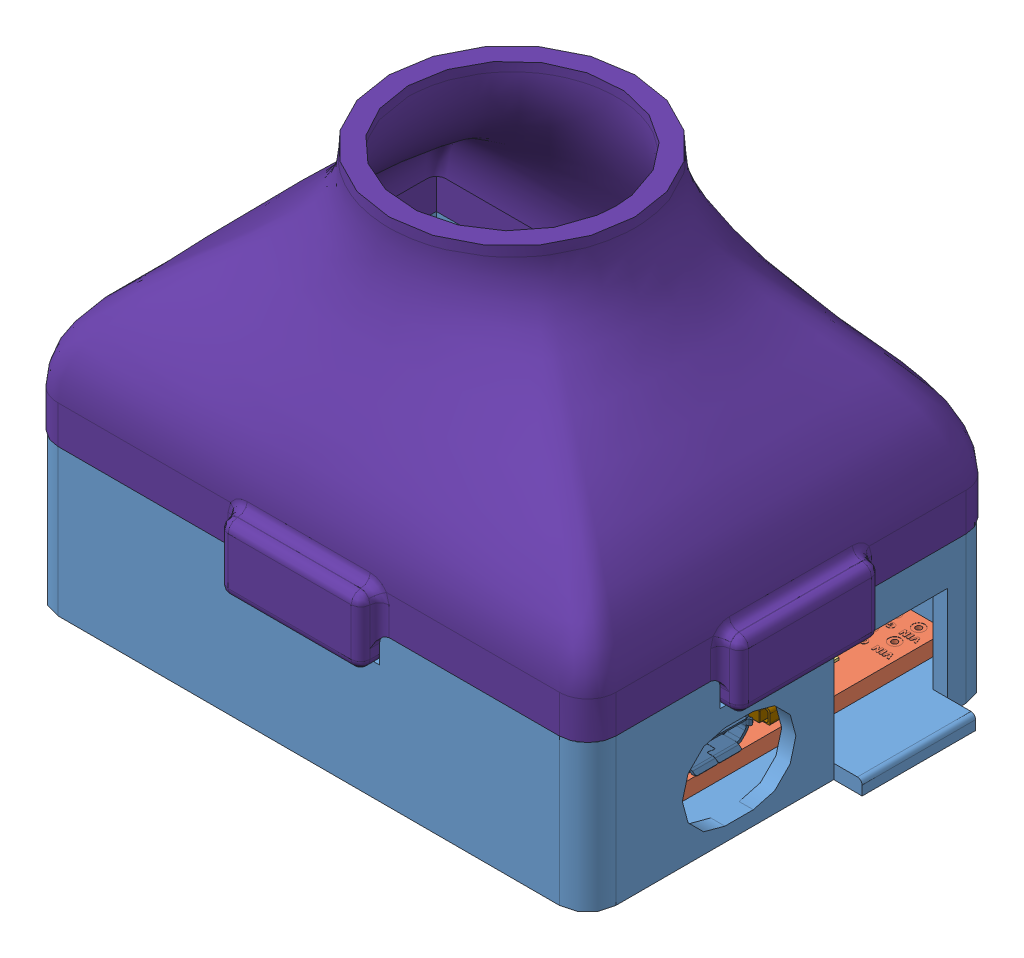
SolidWorks assembly Arduino Case Assembly, configuration Default. Lengths in mm.
Overall size (73 45.5 47).
47 component instances, 17 part files, 8 mates.
Components (placement in the parent):
- Mega 2560 Pro embed Case-1: Mega 2560 Pro embed Case [Default] at origin size (73 15.5 43)
- MEGA 2560 PRO (EMBED)-1: MEGA 2560 PRO (EMBED) [Default] at (0 3.5 0) x (0 0 1) z (0 1 0) size (38 54.09 6.02)
  - MEGA 2560 PRO (EMBED).stp-1: MEGA 2560 PRO (EMBED).stp [Default] at origin size (38 54.09 6.02)
    - Mega 2560 Pro - Board.stp-1: Mega 2560 Pro - Board.stp [Default] at origin size (38 54 1.78)
    - SOT223-3.stp-1: SOT223-3.stp [Default] at (-7.7036 13.3224 1.6256) x (-1 0 0) z (0 0 1) size (6.5 7.07 1.6)
    - SOT223-3.stp-2: SOT223-3.stp [Default] at (-7.5781 23.9617 1.6256) x (-1 0 0) z (0 0 1) size (6.5 7.07 1.6)
    - ATmega2560-16AU.stp-1: ATmega2560-16AU.stp [Default] at (0.2253 -9.3836 1.5256) x (0.707107 -0.707107 0) z (0 0 1) size (16 16 1.21)
    - SOIC -16.stp-1: SOIC -16.stp [Default] at (0.546 8.9647 1.4756) x (0 1 0) z (1 0 0) size (6 1.4 9.9)
    - Crystal Oscillator (SMD).stp-1: Crystal Oscillator (SMD).stp [Default] at (-10.7852 -19.6364 2.54) x (0 -1 0) z (0 0 1) size (13.06 4.55 4.32)
    - Crystal Oscillator (SMD).stp-2: Crystal Oscillator (SMD).stp [Default] at (10.6809 3.6875 2.54) x (0 -1 0) z (0 0 1) size (13.06 4.55 4.32)
    - 1206 Capacitor.stp-1: 1206 Capacitor.stp [Default] at (-3.8106 17.9279 1.6231) x (0 -1 0) z (0 0 1) size (3.2 1.6 1.6)
    - Fuse (1206) - Green.stp-1: Fuse (1206) - Green.stp [Default] at (-0.2207 16.3875 1.6281) x (0 -1 0) z (0 0 1) size (3.28 1.75 0.87)
    - Diode - SMD - DO-214AC.stp-1: Diode - SMD - DO-214AC.stp [Default] at (-1.7706 25.543 1.4756) x (0 -1 0) z (0 0 1) size (5.6 2.95 2.91)
    - USB - Micro.stp-1: USB - Micro.stp [Default] at (2.2104 21.1734 1.3475) x (-1 0 0) z (0 1 0) size (7.92 3.01 5.67)
    - 0603 Capacitor.stp-1: 0603 Capacitor.stp [Default] at (10.7145 18.9901 1.6231) x (0 -1 0) z (0 0 1) size (1.6 0.84 0.84)
    - 0603 Capacitor.stp-2: 0603 Capacitor.stp [Default] at (4.611 3.4374 1.6231) x (0 -1 0) z (0 0 1) size (1.6 0.84 0.84)
    - 0603 Capacitor.stp-3: 0603 Capacitor.stp [Default] at (7.1573 7.8647 1.6231) x (0 1 0) z (0 0 1) size (1.6 0.84 0.84)
    - 0603 Capacitor.stp-4: 0603 Capacitor.stp [Default] at (7.0977 13.4599 1.6231) x (0 1 0) z (0 0 1) size (1.6 0.84 0.84)
    - 0603 Capacitor.stp-5: 0603 Capacitor.stp [Default] at (5.1576 -19.4722 1.6231) x (0 1 0) z (1 0 0) size (1.6 0.84 0.84)
    - 0603 Capacitor.stp-6: 0603 Capacitor.stp [Default] at (-10.8858 1.8771 1.6231) x (0 1 0) z (1 0 0) size (1.6 0.84 0.84)
    - 0603 Capacitor.stp-7: 0603 Capacitor.stp [Default] at (2.9599 3.4697 1.6231) x (0 -1 0) z (0 0 1) size (1.6 0.84 0.84)
    - 0603 Capacitor.stp-8: 0603 Capacitor.stp [Default] at (2.0157 3.7447 1.6231) x (-1 0 0) z (0 0 1) size (1.6 0.84 0.84)
    - 0603 Capacitor.stp-9: 0603 Capacitor.stp [Default] at (-8.0885 -1.9063 1.6231) x (0 1 0) z (1 0 0) size (1.6 0.84 0.84)
    - 0603 Capacitor.stp-10: 0603 Capacitor.stp [Default] at (-3.7884 20.5934 1.6231) x (0 1 0) z (0 0 1) size (1.6 0.84 0.84)
    - 0603 Capacitor.stp-11: 0603 Capacitor.stp [Default] at (-8.8216 3.4762 1.6231) x (0 -1 0) z (0 0 1) size (1.6 0.84 0.84)
    - 0603 Capacitor.stp-12: 0603 Capacitor.stp [Default] at (6.3032 3.4697 2.4613) x (0 -1 0) z (1 0 0) size (1.6 0.84 0.84)
    - 0603 Capacitor.stp-13: 0603 Capacitor.stp [Default] at (-6.2819 -20.9115 1.6231) x (-1 0 0) z (0 1 0) size (1.6 0.84 0.84)
    - 0603 Capacitor.stp-14: 0603 Capacitor.stp [Default] at (-7.8888 -17.889 1.6231) size (1.6 0.84 0.84)
    - 0603 Resistor.stp-1: 0603 Resistor.stp [Default] at (-6.1185 1.9325 1.6231) x (0 1 0) z (0 0 1) size (1.6 0.85 0.56)
    - 0603 Resistor.stp-2: 0603 Resistor.stp [Default] at (-8.697 -1.8307 1.6231) x (0 1 0) z (0 0 1) size (1.6 0.85 0.56)
    - 0603 Resistor.stp-3: 0603 Resistor.stp [Default] at (-10.3133 -1.7908 1.6231) x (0 1 0) z (0 0 1) size (1.6 0.85 0.56)
    - 0603 Resistor.stp-4: 0603 Resistor.stp [Default] at (6.8981 17.2332 1.6231) x (0 1 0) z (0 0 1) size (1.6 0.85 0.56)
    - 0603 Resistor.stp-5: 0603 Resistor.stp [Default] at (-4.1536 1.9449 1.6231) x (0 1 0) z (0 0 1) size (1.6 0.85 0.56)
    - 0603 Resistor.stp-6: 0603 Resistor.stp [Default] at (7.1292 10.6782 1.6231) x (0 1 0) z (0 0 1) size (1.6 0.85 0.56)
    - 0603 Resistor.stp-7: 0603 Resistor.stp [Default] at (5.2754 17.2903 1.6231) x (0 1 0) z (0 0 1) size (1.6 0.85 0.56)
    - 0603 Resistor.stp-8: 0603 Resistor.stp [Default] at (9.8818 17.3443 1.6231) x (0 1 0) z (0 0 1) size (1.6 0.85 0.56)
    - 0603 Resistor.stp-9: 0603 Resistor.stp [Default] at (-11.9263 1.9088 1.6231) x (0 1 0) z (0 0 1) size (1.6 0.85 0.56)
    - 0603 Resistor.stp-10: 0603 Resistor.stp [Default] at (7.18 4.9009 1.6231) x (0 1 0) z (0 0 1) size (1.6 0.85 0.56)
    - 0603 Resistor.stp-11: 0603 Resistor.stp [Default] at (-11.9146 -1.6797 1.6231) x (0 1 0) z (0 0 1) size (1.6 0.85 0.56)
    - 0603 Resistor.stp-12: 0603 Resistor.stp [Default] at (-6.3495 -18.5603 1.6231) x (-1 0 0) z (0 0 1) size (1.6 0.85 0.56)
    - LED - 0603 - Blue.stp-1: LED - 0603 - Blue.stp [Default] at (7.1908 -19.2239 1.6256) x (0 1 0) z (0 0 1) size (1.63 0.73 0.83)
    - LED_-_Vishay_-_6063_-_Green.stp-1: LED_-_Vishay_-_6063_-_Green.stp [Default] at (10.6783 -18.0475 1.5956) x (0 -1 0) z (0 0 1) size (1.63 0.73 0.83)
    - LED - 0603 - Blue.stp-2: LED - 0603 - Blue.stp [Default] at (9.0246 -17.9783 1.6256) x (0 -1 0) z (0 0 1) size (1.63 0.73 0.83)
    - 1206 Fuse.stp-1: 1206 Fuse.stp [Default] at (1.6964 17.9461 1.6231) x (0 -1 0) z (0 0 1) size (3.2 1.6 0.53)
    - SWT-32.stp-1: SWT-32.stp [Default] at (15.7781 21.6695 1.6256) x (0 1 0) z (0 0 1) size (8 6.4 2.9)
    - LED - 0603 - Blue.stp-3: LED - 0603 - Blue.stp [Default] at (12.5463 -18.1103 1.6256) x (0 -1 0) z (0 0 1) size (1.63 0.73 0.83)
- Arduino cables-1: Arduino cables [Default] at (0 15.5 0) x (1 0 0) z (0 1 0) size (63 47 33)
Mates (geometry in assembly coordinates):
- Coincident1: coordinate: point of Mega 2560 Pro embed Case-1
- Distance1: distance = 1 mm anti-aligned: plane of MEGA 2560 PRO (EMBED)-1/MEGA 2560 PRO (EMBED).stp-1/Mega 2560 Pro - Board.stp-1 through (27 5.1256 -19) normal (1 0 0); plane of Mega 2560 Pro embed Case-1 through (28 15.5 0) normal (-1 0 0)
- Distance2: distance = 1 mm anti-aligned: plane of MEGA 2560 PRO (EMBED)-1/MEGA 2560 PRO (EMBED).stp-1/Mega 2560 Pro - Board.stp-1 through (-27 5.1256 -19) normal (0 0 -1); plane of Mega 2560 Pro embed Case-1 through (0 15.5 -20) normal (0 0 1)
- Distance3: distance = 2 mm anti-aligned: plane of MEGA 2560 PRO (EMBED)-1/MEGA 2560 PRO (EMBED).stp-1/Mega 2560 Pro - Board.stp-1 through (0 3.5 0) normal (0 -1 0); plane of Mega 2560 Pro embed Case-1 through (0 1.5 0) normal (0 1 0)
- InPlace1: in place: plane of Mega 2560 Pro embed Case-1 through (0 15.5 0) normal (0 1 0); plane of Arduino cables-1 through (0 15.5 0) normal (0 1 0); moOrthogonalPlaneRef_w of Mega 2560 Pro embed Case-1 through (0 15.5 0) normal (0 1 0); plane of Arduino cables-1 through (0 15.5 0) normal (0 0 -1); plane of Mega 2560 Pro embed Case-1 through (0 15.5 0) normal (0 1 0); plane of Arduino cables-1 through (0 15.5 0) normal (1 0 0); plane of Mega 2560 Pro embed Case-1 through (0 15.5 0) normal (0 1 0); unknown of Arduino cables-1
- Coincident5: coincident aligned: plane of Mega 2560 Pro embed Case-1; plane of Arduino cables-1
- Coincident6: coincident aligned: moOrthogonalPlaneRef_w of Mega 2560 Pro embed Case-1 through (0 15.5 0) normal (0 0 -1); plane of Arduino cables-1 through (0 15.5 0) normal (0 0 -1)
- Coincident7: coincident anti-aligned: moOrthogonalPlaneRef_w of Mega 2560 Pro embed Case-1 through (0 15.5 0) normal (-1 0 0); plane of Arduino cables-1 through (0 15.5 0) normal (1 0 0)
